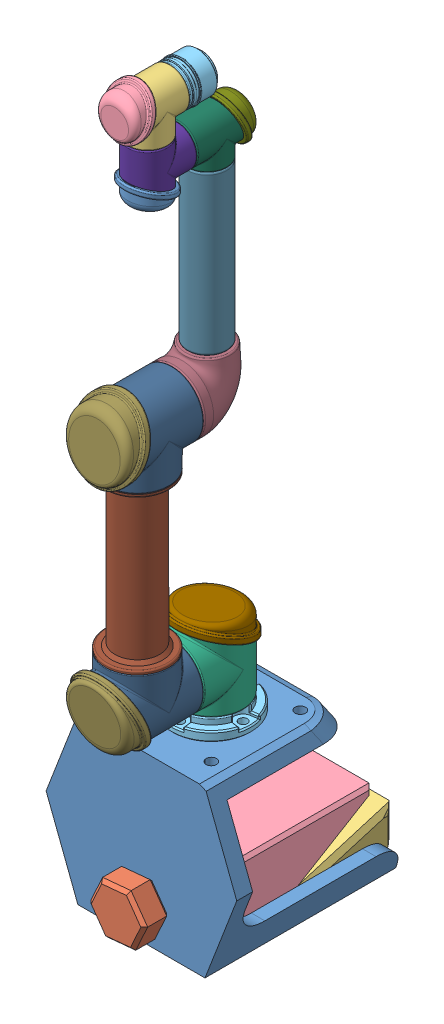
SolidWorks assembly 机械臂手机支架, configuration 默认. Lengths in mm.
Overall size (60 236.23 78.63).
30 component instances, 25 part files, 56 mates.
Components (placement in the parent):
- 台钳-1: 台钳 [默认] at origin size (60 55.6 70.56)
  - 台钳架-1: 台钳架 [默认] at origin size (60 55.17 60)
  - 螺杆-1: 螺杆 [默认] at (0 -15 0) x (0.416104 0.909317 0) z (0 0 1) size (18 15.59 53)
  - 滑块-1: 滑块 [默认] at (0 -15 -55.8903) size (45 17.4 31.72)
  - 桌子-1: 桌子 [默认] at (1.7431 21 -55) x (-1 0 0) z (0 -1 0) size (200 100 20) (hidden)
  - 顶块-1: 顶块 [默认] at (0 -5.0342 -42.5) x (-1 0 0) z (0 0 -1) size (35.2 18 50)
- base-1: base [默认] at (0 26 -22) x (1 0 0) z (0 1 0) size (25 25 6.93)
- J1-1: J1 [默认] at (0 42.5 -22) x (0.008711 0 0.999962) z (0 -1 0) size (23.75 20.59 23.04)
- 螺钉-大-1: 螺钉-大 [默认] at (0 35 -22) x (1 0 0) z (0 1 0) size (14.8 14.8 15.1)
- 螺钉-大-长轴-1: 螺钉-大-长轴 [默认] at (0.135 42 -6.5006) x (0.999962 0 -0.008711) z (0.008711 0 0.999962) size (14.8 14.8 25.14)
- J1-盖子-1: J1-盖子 [默认] at (0 51.5018 -22) x (0.008711 0 0.999962) z (-0.999962 0 0.008711) size (22.2 11.37 22.2)
- 扳手-1: 扳手 [默认] at (0 44.8 -22) x (1 0 0) z (0 -1 0) size (11 11 25) (hidden)
- J2-1: J2 [默认] at (0.2091 42 1.9991) x (0 1 0) z (-0.008711 0 -0.999962) size (22.75 20.59 23.04)
- J2_link-1: J2_link [默认] at (0.2047 79.1 1.4991) x (0 1 0) z (0.008711 0 0.999962) size (79.01 20 20)
- J2-2: J2 [默认] at (0.2047 116.2 1.9991) x (0 -1 0) z (0 0 -1) size (22.75 20.59 23.04)
- J2-盖子-1: J2-盖子 [默认] at (0.2879 42 11.0537) x (0 1 0) z (0.999962 0 -0.008711) size (22.2 11.37 22.2)
- 螺钉-大-长轴-2: 螺钉-大-长轴 [默认] at (0.2047 116.2 -6.5009) x (0.794262 -0.607575 0) z (0 0 1) size (14.8 14.8 25.14)
- J2-盖子-2: J2-盖子 [默认] at (0.2047 116.2 11.0541) x (0 -1 0) z (-1 0 0) size (22.2 11.37 22.2)
- J3-1: J3 [默认] at (0.2047 116.2 -11.0009) x (0 1 0) z (0 0 -1) size (21.85 20.53 19.74)
- J3-link-1: J3-link [默认] at (0.2047 127.7 -20.4509) x (0 0 -1) z (0 1 0) size (12.5 12.5 70.04)
- J3_-1: J3_ [默认] at (0.2047 185.7 -19.9509) x (0 -1 0) z (0 0 1) size (14.27 12.63 17.39)
- J3-盖子-1: J3-盖子 [默认] at (0.2047 185.7 -25.7684) x (0 -1 0) z (1 0 0) size (14.7 8.18 14.7)
- J4-1: J4 [默认] at (0.2047 185.2 -1.7009) x (0 0 -1) z (0 1 0) size (16.77 12.63 15.39)
- 螺钉-小-长轴-1: 螺钉-小-长轴 [默认] at (0.2047 185.7 -13.7009) x (-0.870356 -0.492423 0) z (0 0 -1) size (8.2 8.2 21.84)
- J4-盖子-1: J4-盖子 [默认] at (0.2047 180.276 -1.7009) x (0 0 -1) z (-1 0 0) size (14.7 8.18 14.7)
- 螺钉-小-1: 螺钉-小 [默认] at (0.2047 190.45 -1.7009) x (1 0 0) z (0 -1 0) size (8.2 8.2 12.59)
- J5-1: J5 [默认] at (0.2047 202.45 -1.2009) x (0 -1 0) z (0 0 -1) size (16.77 12.63 15.39)
- 螺钉-小-2: 螺钉-小 [默认] at (0.2047 202.45 -6.4509) size (8.2 8.2 12.59)
- J5-盖子-1: J5-盖子 [默认] at (0.2047 202.45 3.6167) x (0 -1 0) z (-1 0 0) size (14.7 8.18 14.7)
- J6-1: J6 [默认] at (0.2047 202.45 -17.5509) x (0 0 1) z (-1 0 0) size (10.8 12.9 12.9)
Mates (geometry in assembly coordinates):
- 重合1: coincident anti-aligned: plane of 台钳-1/台钳架-1 through (-20 26 -5) normal (0 1 0); plane of base-1 through (0 26 -22) normal (0 -1 0)
- 同心1: concentric anti-aligned: cylinder of 台钳-1/台钳架-1 through (10 -26.001 -22) axis (0 1 0) radius 1.65; cylinder of base-1 through (10 28 -22) axis (0 -1 0) radius 1.35
- 同心2: concentric anti-aligned: cylinder of 台钳-1/台钳架-1 through (-10 -26.001 -22) axis (0 1 0) radius 1.65; cylinder of base-1 through (-10 28 -22) axis (0 -1 0) radius 1.35
- 重合2: coincident anti-aligned: plane of base-1 through (0 31 -27) normal (0 1 0); plane of J1-1 through (0 31 -22) normal (0 -1 0)
- 同心3: concentric anti-aligned: cylinder of base-1 through (0 28 -22) axis (0 -1 0) radius 12.5; cylinder of J1-1 through (0 31 -22) axis (0 1 0) radius 10
- 重合8: coincident anti-aligned: plane of J1-1 through (0 35 -22) normal (0 1 0); plane of 螺钉-大-1 through (0 35 -22) normal (0 -1 0)
- 同心6: concentric anti-aligned: cylinder of J1-1 through (0 35 -22) axis (0 1 0) radius 7.5; cylinder of 螺钉-大-1 through (0 37.8 -22) axis (0 -1 0) radius 7.4
- 距离1: distance = 0.05 mm anti-aligned: plane of J1-1 through (0.0015 49.2905 -21.829) normal (-0.002979 0.939693 -0.342007); plane of J1-盖子-1 through (14.9023 45.2224 -33.2824) normal (0.002979 -0.939693 0.342007)
- 同心10: concentric anti-aligned: cylinder of J1-1 through (0 31 -22) axis (0 1 0) radius 10; cylinder of J1-盖子-1 through (0 56.5018 -22) axis (0 -1 0) radius 10
- 重合14: coincident anti-aligned: plane of 螺钉-大-1 through (0 37.8 -22) normal (0 1 0); plane of 扳手-1 through (0 37.8 -22) normal (0 -1 0)
- 同心11: concentric aligned: cylinder of J1-1 through (0 35 -22) axis (0 1 0) radius 7.5; cylinder of 扳手-1 through (0 37.8 -22) axis (0 1 0) radius 5.5
- 重合15: coincident anti-aligned: plane of J1-1 through (0.1089 42 -9.5005) normal (0.008711 0 0.999962); plane of J2-1 through (0.1089 42 -9.5005) normal (-0.008711 0 -0.999962)
- 同心12: concentric anti-aligned: cylinder of J1-1 through (0.1089 42 -9.5005) axis (-0.008711 0 -0.999962) radius 10; cylinder of J2-1 through (0.1089 42 -9.5005) axis (0.008711 0 0.999962) radius 10
- 重合16: coincident anti-aligned: plane of 螺钉-大-长轴-1 through (0.135 42 -6.5006) normal (-0.008711 0 -0.999962); plane of J2-1 through (0.135 42 -6.5006) normal (0.008711 0 0.999962)
- 重合17: coincident anti-aligned: plane of J2-1 through (0.2047 54.5 1.4991) normal (0 1 0); plane of J2_link-1 through (-4.7951 54.5 1.5427) normal (0 -1 0)
- 同心13: concentric aligned: cylinder of J2-1 through (0.2047 54.5 1.4991) axis (0 -1 0) radius 10; cylinder of J2_link-1 through (0.2047 46.7681 1.4991) axis (0 -1 0) radius 7
- 同心14: concentric anti-aligned: cylinder of 螺钉-大-长轴-1 through (0.25 42 6.6989) axis (-0.008711 0 -0.999962) radius 3.5; cylinder of J2_link-1 through (0.1394 42 -6.0006) axis (0.008711 0 0.999962) radius 3.6
- 重合18: coincident anti-aligned: plane of J2_link-1 through (-4.7951 103.7 1.5427) normal (0 1 0); plane of J2-2 through (0.2047 103.7 1.4991) normal (0 -1 0)
- 同心15: concentric anti-aligned: cylinder of J2_link-1 through (0.2047 46.7681 1.4991) axis (0 -1 0) radius 7; cylinder of J2-2 through (0.2047 103.7 1.4991) axis (0 1 0) radius 10
- 同心16: concentric anti-aligned: cylinder of J2-1 through (0.1089 42 -9.5005) axis (0.008711 0 0.999962) radius 10; cylinder of J2-盖子-1 through (0.3315 42 16.0535) axis (-0.008711 0 -0.999962) radius 10
- 距离2: distance = 0.1 mm anti-aligned: plane of J2-盖子-1 through (-14.7662 30.8479 4.9052) normal (-0.008186 0.34202 -0.939657); plane of J2-1 through (0.2682 42.171 8.7893) normal (0.008186 -0.34202 0.939657)
- 重合20: coincident anti-aligned: plane of J2-2 through (0.2047 116.2 -6.5009) normal (0 0 1); plane of 螺钉-大-长轴-2 through (0.2047 116.2 -6.5009) normal (0 0 -1)
- 同心17: concentric anti-aligned: cylinder of J2-2 through (0.2047 116.2 -6.5009) axis (0 0 1) radius 7.5; cylinder of 螺钉-大-长轴-2 through (0.2047 116.2 -3.7009) axis (0 0 -1) radius 7.4
- 平行1: parallel anti-aligned: plane of J2-2 through (0.2047 116.2 -9.5009) normal (0 0 -1)
- 同心18: concentric anti-aligned: cylinder of J2-2 through (0.2047 116.2 -9.5009) axis (0 0 1) radius 10; cylinder of J2-盖子-2 through (0.2047 116.2 16.0541) axis (0 0 -1) radius 10
- 距离3: distance = 0.1 mm anti-aligned: plane of J2-盖子-2 through (15.2047 127.3521 4.7747) normal (0 -0.34202 -0.939693); plane of J2-2 through (0.2047 116.029 8.7896) normal (0 0.34202 0.939693)
- 重合23: coincident anti-aligned: plane of J2-2 through (0.2047 116.2 -9.5009) normal (0 0 -1); plane of J3-1 through (0.2047 116.2 -9.5009) normal (0 0 1)
- 同心19: concentric aligned: cylinder of J2-2 through (0.2047 116.2 -9.5009) axis (0 0 1) radius 10; cylinder of J3-1 through (0.2047 116.2 -12.5009) axis (0 0 1) radius 10
- 平行2: parallel aligned: plane of J2_link-1 through (-9.7949 55.5 1.5862) normal (0 1 0)
- 同心20: concentric anti-aligned: cylinder of J3-1 through (0.2047 115.7 -20.4509) axis (0 1 0) radius 4.25; cylinder of J3-link-1 through (0.2047 177.7 -20.4509) axis (0 -1 0) radius 6.25
- 重合25: coincident anti-aligned: plane of J3-1 through (0.2047 127.7 -20.4509) normal (0 1 0); plane of J3-link-1 through (0.2047 127.7 -20.4509) normal (0 -1 0)
- 平行3: parallel aligned: plane of J3-link-1 through (0.2047 177.7 -20.4509) normal (0 1 0)
- 同心21: concentric anti-aligned: cylinder of J3-1 through (0.2047 119.7 -25.4509) axis (0 0 1) radius 2.5; cylinder of J3-link-1 through (0.2047 119.7 -15.4509) axis (0 0 -1) radius 2.6
- 重合27: coincident anti-aligned: plane of J3-link-1 through (0.2047 177.7 -20.4509) normal (0 1 0); plane of J3_-1 through (0.2047 177.7 -20.4509) normal (0 -1 0)
- 同心22: concentric anti-aligned: cylinder of J3-link-1 through (0.2047 177.7 -20.4509) axis (0 -1 0) radius 6.25; cylinder of J3_-1 through (0.2047 177.7 -20.4509) axis (0 1 0) radius 6.25
- 平行4: parallel aligned: plane of J3_-1 through (0.2047 185.7 -11.2009) normal (0 0 1)
- 同心23: concentric anti-aligned: cylinder of J3_-1 through (0.2047 185.7 -11.2009) axis (0 0 -1) radius 6.25; cylinder of J3-盖子-1 through (0.2047 185.7 -30.7684) axis (0 0 1) radius 6.25
- 重合28: coincident anti-aligned: plane of J3_-1 through (0.2047 185.529 -25.3562) normal (0 0.34202 -0.939693); plane of J3-盖子-1 through (-14.7953 193.05 -22.6188) normal (0 -0.34202 0.939693)
- 重合29: coincident anti-aligned: plane of J3_-1 through (0.2047 185.7 -11.2009) normal (0 0 1); plane of J4-1 through (0.2047 185.7 -11.2009) normal (0 0 -1)
- 同心24: concentric anti-aligned: cylinder of J3_-1 through (0.2047 185.7 -11.2009) axis (0 0 -1) radius 6.25; cylinder of J4-1 through (0.2047 185.7 -11.2009) axis (0 0 1) radius 6.25
- 平行5: parallel aligned: plane of J4-1 through (0.2047 192.95 -1.7009) normal (0 1 0)
- 同心25: concentric anti-aligned: cylinder of J3_-1 through (0.2047 185.7 -11.2009) axis (0 0 -1) radius 6.25; cylinder of 螺钉-小-长轴-1 through (0.2047 185.7 -24.1009) axis (0 0 1) radius 2.5
- 重合32: coincident anti-aligned: plane of J3_-1 through (0.2047 185.7 -13.7009) normal (0 0 -1); plane of 螺钉-小-长轴-1 through (0.2047 185.7 -13.7009) normal (0 0 1)
- 同心26: concentric anti-aligned: cylinder of J4-1 through (0.2047 192.95 -1.7009) axis (0 -1 0) radius 6.25; cylinder of J4-盖子-1 through (0.2047 175.276 -1.7009) axis (0 1 0) radius 6.25
- 距离4: distance = 0.1 mm anti-aligned: plane of J4-盖子-1 through (15.2047 183.4257 5.6491) normal (0 0.939693 -0.34202); plane of J4-1 through (0.2047 180.7947 -1.8719) normal (0 -0.939693 0.34202)
- 同心27: concentric anti-aligned: cylinder of J4-1 through (0.2047 190.45 -1.7009) axis (0 -1 0) radius 4.25; cylinder of 螺钉-小-1 through (0.2047 188.05 -1.7009) axis (0 1 0) radius 4.1
- 重合34: coincident anti-aligned: plane of J4-1 through (0.2047 190.45 -1.7009) normal (0 -1 0); plane of 螺钉-小-1 through (0.2047 190.45 -1.7009) normal (0 1 0)
- 重合35: coincident anti-aligned: plane of J4-1 through (0.2047 192.95 -1.7009) normal (0 1 0); plane of J5-1 through (0.2047 192.95 -1.7009) normal (0 -1 0)
- 同心28: concentric anti-aligned: cylinder of J4-1 through (0.2047 192.95 -1.7009) axis (0 -1 0) radius 6.25; cylinder of J5-1 through (0.2047 192.95 -1.7009) axis (0 1 0) radius 6.25
- 平行8: parallel anti-aligned: plane of J5-1 through (0.2047 202.45 -8.9509) normal (0 0 -1)
- 同心29: concentric anti-aligned: cylinder of J5-1 through (0.2047 202.45 -8.9509) axis (0 0 1) radius 6.25; cylinder of 螺钉-小-2 through (0.2047 202.45 -4.0509) axis (0 0 -1) radius 4.1
- 重合36: coincident anti-aligned: plane of J5-1 through (0.2047 202.45 -6.4509) normal (0 0 1); plane of 螺钉-小-2 through (0.2047 202.45 -6.4509) normal (0 0 -1)
- 同心30: concentric anti-aligned: cylinder of J5-1 through (0.2047 202.45 -8.9509) axis (0 0 1) radius 6.25; cylinder of J5-盖子-1 through (0.2047 202.45 8.6167) axis (0 0 -1) radius 6.25
- 重合37: coincident anti-aligned: plane of J5-1 through (0.2047 202.279 3.2044) normal (0 0.34202 0.939693); plane of J5-盖子-1 through (15.2047 209.8 0.467) normal (0 -0.34202 -0.939693)
- 重合38: coincident anti-aligned: plane of J5-1 through (0.2047 202.45 -8.9509) normal (0 0 -1); plane of J6-1 through (0.2047 208.45 -8.9509) normal (0 0 1)
- 同心31: concentric anti-aligned: cylinder of J5-1 through (0.2047 202.45 -8.9509) axis (0 0 1) radius 6.25; cylinder of J6-1 through (0.2047 202.45 -37.2319) axis (0 0 -1) radius 6.25
